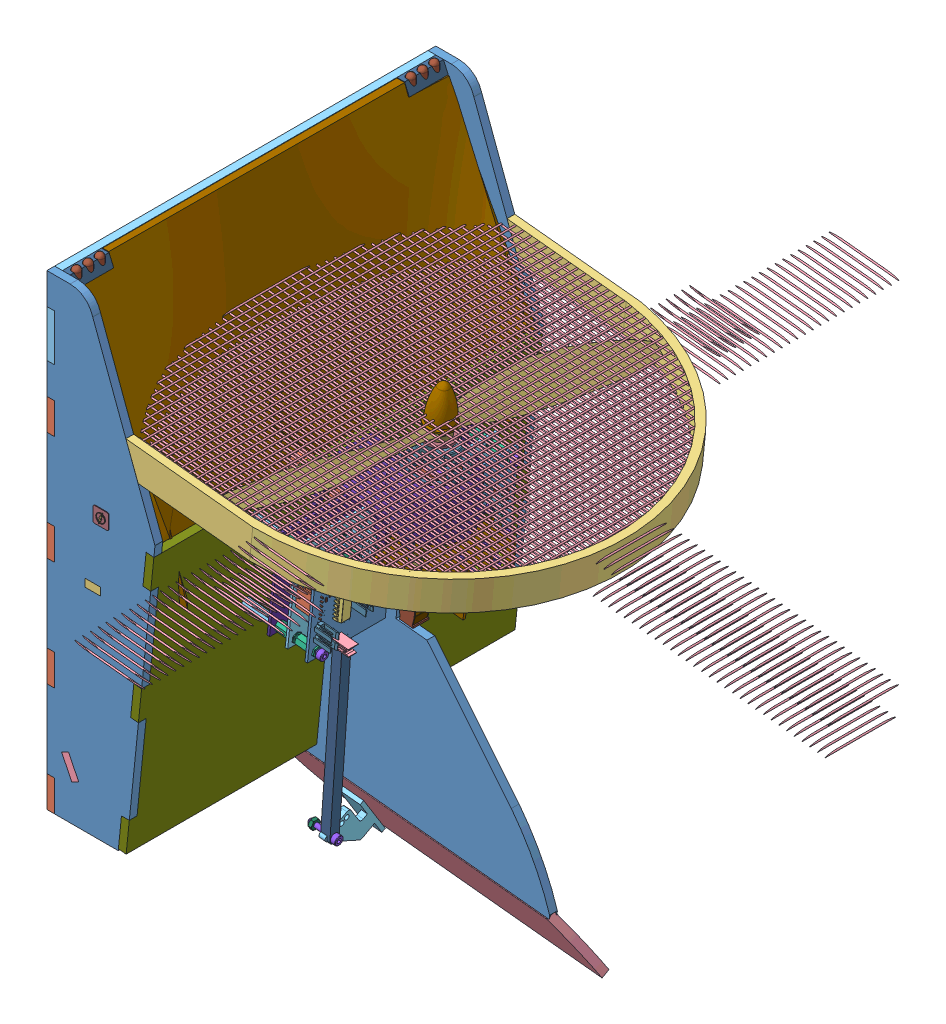
SolidWorks assembly AssTotaleSimu8, configuration Défaut. Lengths in mm.
Overall size (253.25 382.9 251.6).
1718 component instances, 230 part files, 11 mates.
Components (placement in the parent):
- AssStructSimu-1: AssStructSimu [Défaut] at (-125.7658 -1.8483 624.6548) x (1 0 0) z (0 0 -1) size (253.25 324.59 251.6)
  - AssBase-1: AssBase [Défaut] at (36.5482 -71.0398 34.0612) size (86.08 302.3 251.6)
    - AssD-1: AssD [Défaut] at (39.0992 31.0201 8.5) size (69.5 300 22)
      - P1-1: P1 [Défaut] at (-95.5819 194.6656 377.5) size (69.5 300 5)
      - P5-1: P5 [Défaut] at (-100.5819 -35.3344 360.5) x (0 1 0) z (1 0 0) size (230 22 5)
    - AssG-1: AssG [Défaut] at (39.0992 31.0201 -236.5) size (69.5 300 22)
      - P1-1: P1 [Défaut] at (-95.5819 194.6656 377.5) size (69.5 300 5)
      - P5-1: P5 [Défaut] at (-95.5819 -35.3344 399.5) x (0 1 0) z (-1 0 0) size (230 22 5)
    - P7-1: P7 [Défaut] at (-1.4828 89.6857 370.5) x (0 0 -1) z (0 -1 0) size (250 54.5 5)
    - P4-1: P4 [Défaut] at (-63.2363 165.9323 386) x (0 0 -1) z (0.898794 -0.438371 0) size (250 60.5 66.27)
    - P3-1: P3 [Défaut] at (-56.4828 -74.3143 146) x (0 0 1) z (-1 0 0) size (250 70 5)
    - P4b-1: P4b [Défaut] at (-58.7423 163.7404 190) x (0 0 1) z (0.438371 0.898794 0) size (152 56 2)
    - battery-1: battery [Défaut] at (-39.0156 204.1861 197.5) x (0 0 1) z (0.898794 -0.438371 0) size (137 43 30)
    - socket head cap screw 4762_din-1: socket head cap screw 4762_din [EN ISO 4762 M3 x 10 - 10N] at (-27.7008 145.2627 193) x (0.438371 0.898794 0) z (0 0 -1) size (13 5.5 5.5)
    - socket head cap screw 4762_din-2: socket head cap screw 4762_din [EN ISO 4762 M3 x 10 - 10N] at (-27.7008 145.2627 339) x (0.438371 0.898794 0) z (-0.791285 0.385936 -0.474259) size (13 5.5 5.5)
    - socket head cap screw 4762_din-3: socket head cap screw 4762_din [EN ISO 4762 M3 x 10 - 10N] at (-42.0815 152.2766 339) x (0.438371 0.898794 0) z (-0.001489 0.000726 -0.999999) size (13 5.5 5.5)
    - socket head cap screw 4762_din-4: socket head cap screw 4762_din [EN ISO 4762 M3 x 10 - 10N] at (-42.0815 152.2766 193) x (0.438371 0.898794 0) z (-0.031331 0.015281 -0.999392) size (13 5.5 5.5)
    - P11-1: P11 [Défaut] at (-57.5734 -73.9703 146.7843) x (0.005072 0 0.999987) z (0.006197 0.999981 -0.000031) size (240 65 164)
    - AssPhare-1: AssPhare [Défaut] at (-52.8518 -67.6977 411) x (0 1 0) z (0 0 -1) size (35.8 8 25)
      - piece_led-1: piece_led [Défaut] at (-6.6166 -3.631 25) size (7 8 25)
      - LED 5mm-1: LED 5mm [Valor predeterminado] at (-0.1166 0.369 30) x (0 0 1) z (-1 0 0) size (10.06 6 40.8)
      - LED 5mm-2: LED 5mm [Valor predeterminado] at (-0.1166 0.369 37.5) x (0 0 1) z (-1 0 0) size (10.06 6 40.8)
      - LED 5mm-3: LED 5mm [Valor predeterminado] at (-0.1166 0.369 45) x (0 0 1) z (-1 0 0) size (10.06 6 40.8)
    - AssPhare-2: AssPhare [Défaut] at (-52.8518 -67.6977 196) x (0 1 0) z (0 0 -1) size (35.8 8 25)
      - piece_led-1: piece_led [Défaut] at (-6.6166 -3.631 25) size (7 8 25)
      - LED 5mm-1: LED 5mm [Valor predeterminado] at (-0.1166 0.369 30) x (0 0 1) z (-1 0 0) size (10.06 6 40.8)
      - LED 5mm-2: LED 5mm [Valor predeterminado] at (-0.1166 0.369 37.5) x (0 0 1) z (-1 0 0) size (10.06 6 40.8)
      - LED 5mm-3: LED 5mm [Valor predeterminado] at (-0.1166 0.369 45) x (0 0 1) z (-1 0 0) size (10.06 6 40.8)
    - AssLogo-1: AssLogo [Défaut] at (-27.8835 45.1673 148.1054) x (-1 0 0) z (0 0 -1) size (10 10 0.8)
      - logo1-1: logo1 [Défaut] at (-6.5271 -4.4734 6.5054) size (5.8 7.71 0.4)
      - logo2-1: logo2 [Défaut] at (-6.4007 -4.4815 7.1054) size (10 10 0.4)
    - AssLogo-2: AssLogo [Défaut] at (-25.082 45.1673 383.8946) size (10 10 0.8)
      - logo1-1: logo1 [Défaut] at (-6.5271 -4.4734 6.5054) size (5.8 7.71 0.4)
      - logo2-1: logo2 [Défaut] at (-6.4007 -4.4815 7.1054) size (10 10 0.4)
    - support2-1: support2 [Défaut] at (-61.5648 191.7124 276) x (-0.017452 -0.999848 0) z (0.999848 -0.017452 0) size (75 20 10)
    - socket head cap screw 4762_din-5: socket head cap screw 4762_din [EN ISO 4762 M3 x 5 - 5N] at (-61.652 186.7132 269.3333) x (0.999848 -0.017452 0) z (-0.002158 -0.123615 0.992328) size (8 5.5 5.5)
    - socket head cap screw 4762_din-6: socket head cap screw 4762_din [EN ISO 4762 M3 x 5 - 5N] at (-61.652 186.7132 262.6667) x (0.999848 -0.017452 0) z (0 0 1) size (8 5.5 5.5)
    - socket head cap screw 4762_din-7: socket head cap screw 4762_din [EN ISO 4762 M3 x 25 - 18N] at (-55.2963 121.0922 253) x (0 0 1) z (-1 0 0) size (28 5.5 5.5)
    - hex nut style 1 gradeab_din-1: hex nut style 1 gradeab_din [Hexagon Nut ISO 4032 - M3 - W - N] at (-55.2963 121.0922 276) x (-0.923728 -0.383049 0) z (0 0 -1) size (5.5 6.35 2.4)
  - AssToitMot-1: AssToitMot [Défaut] at (-168.5238 43.6961 238.494) x (0 0 -1) z (0.9948 0.101852 0) size (250 207.5 205)
    - AssToit-1: AssToit [Défaut] at (-23.0702 -16.5789 -3.7148) size (250 207.5 205)
      - P8-1: P8 [Défaut] at (-38.4971 122.5921 203.5) size (250 175 5)
      - P12-1: P12 [Défaut] at (-60.4971 -63.4079 265.5) x (1 0 0) z (0 -1 0) size (47.03 76.64 55)
      - P13-1: P13 [Défaut] at (-35.9971 -52.8579 208.5) x (0 0 1) z (-1 0 0) size (64 15.55 5)
      - P10_2-1: P10_2 [Défaut] at (-35.9971 111.5921 171) x (0 0 1) z (-1 0 0) size (188.5 117.6 5)
    - Parallax-Servo_DUMMY-1: Parallax-Servo_DUMMY [Défaut] at (-61.6002 -51.5207 216.6662) x (1 0 0) z (0 1 0) size (20.07 42.67 55.64)
    - socket head cap screw 4762_din-1: socket head cap screw 4762_din [EN ISO 4762 M2.5 x 5 - 5N] at (-51.9272 -76.4868 259.2852) x (0 -1 0) z (-0.546944 0 0.837169) size (7.5 4.5 4.5)
    - socket head cap screw 4762_din-2: socket head cap screw 4762_din [EN ISO 4762 M2.5 x 5 - 5N] at (-61.5672 -76.4868 268.9252) x (0 -1 0) z (-0.546944 0 0.837169) size (7.5 4.5 4.5)
    - socket head cap screw 4762_din-3: socket head cap screw 4762_din [EN ISO 4762 M2.5 x 5 - 5N] at (-71.2072 -76.4868 259.2852) x (0 -1 0) z (-0.546944 0 0.837169) size (7.5 4.5 4.5)
    - socket head cap screw 4762_din-4: socket head cap screw 4762_din [EN ISO 4762 M2.5 x 5 - 5N] at (-61.5672 -76.4868 249.6452) x (0 -1 0) z (-0.546944 0 0.837169) size (7.5 4.5 4.5)
    - AssPhare-1: AssPhare [Défaut] at (8.4328 83.3966 196.1542) x (0 -1 0) z (1 0 0) size (35.8 8 25)
      - piece_led-1: piece_led [Défaut] at (-6.6166 -3.631 25) size (7 8 25)
      - LED 5mm-1: LED 5mm [Valor predeterminado] at (-0.1166 0.369 30) x (0 0 1) z (-1 0 0) size (10.06 6 40.8)
      - LED 5mm-2: LED 5mm [Valor predeterminado] at (-0.1166 0.369 37.5) x (0 0 1) z (-1 0 0) size (10.06 6 40.8)
      - LED 5mm-3: LED 5mm [Valor predeterminado] at (-0.1166 0.369 45) x (0 0 1) z (-1 0 0) size (10.06 6 40.8)
    - AssPhare-2: AssPhare [Défaut] at (-206.5672 83.3966 196.1542) x (0 -1 0) z (1 0 0) size (35.8 8 25)
      - piece_led-1: piece_led [Défaut] at (-6.6166 -3.631 25) size (7 8 25)
      - LED 5mm-1: LED 5mm [Valor predeterminado] at (-0.1166 0.369 30) x (0 0 1) z (-1 0 0) size (10.06 6 40.8)
      - LED 5mm-2: LED 5mm [Valor predeterminado] at (-0.1166 0.369 37.5) x (0 0 1) z (-1 0 0) size (10.06 6 40.8)
      - LED 5mm-3: LED 5mm [Valor predeterminado] at (-0.1166 0.369 45) x (0 0 1) z (-1 0 0) size (10.06 6 40.8)
    - socket head cap screw 4762_din-5: socket head cap screw 4762_din [EN ISO 4762 M3 x 10 - 10N] at (-67.0672 -22.9368 210.2852) x (0 0 -1) z (1 0 0) size (13 5.5 5.5)
    - socket head cap screw 4762_din-6: socket head cap screw 4762_din [EN ISO 4762 M3 x 10 - 10N] at (-56.0672 -72.9868 210.2852) x (0 0 -1) z (1 0 0) size (13 5.5 5.5)
    - socket head cap screw 4762_din-7: socket head cap screw 4762_din [EN ISO 4762 M3 x 10 - 10N] at (-67.0672 -72.9868 210.2852) x (0 0 -1) z (1 0 0) size (13 5.5 5.5)
    - socket head cap screw 4762_din-8: socket head cap screw 4762_din [EN ISO 4762 M3 x 10 - 10N] at (-56.0672 -22.9368 210.2852) x (0 0 -1) z (1 0 0) size (13 5.5 5.5)
    - hex nut style 1 gradeab_din-1: hex nut style 1 gradeab_din [Hexagon Nut ISO 4032 - M3 - W - N] at (-67.0672 -72.9868 197.3852) x (-0.923728 -0.383049 0) z (0 0 -1) size (5.5 6.35 2.4)
    - hex nut style 1 gradeab_din-2: hex nut style 1 gradeab_din [Hexagon Nut ISO 4032 - M3 - W - N] at (-56.0672 -72.9868 199.7852) size (5.5 6.35 2.4)
    - hex nut style 1 gradeab_din-3: hex nut style 1 gradeab_din [Hexagon Nut ISO 4032 - M3 - W - N] at (-67.0672 -22.9368 199.7852) size (5.5 6.35 2.4)
    - hex nut style 1 gradeab_din-4: hex nut style 1 gradeab_din [Hexagon Nut ISO 4032 - M3 - W - N] at (-56.0672 -22.9368 199.7852) size (5.5 6.35 2.4)
  - AssProtec-1: AssProtec [Défaut] at (86.6746 190.4649 284.6351) x (0 0 -1) z (0.101852 -0.9948 0) size (250 237.46 20)
    - protec3c-1: protec3c [Défaut] at (-140.4261 -87.7568 240) size (250 197 20)
    - AssGrillage-1: AssGrillage [Défaut] at (-370.4609 -132.5428 258.3161) x (0 0 -1) z (1 0 0) size (2.02 237.05 250)
      - barreau-1: barreau [Défaut] at (-1.1839 0.254 200) size (1 1 400)
      - barreau-3: barreau [Défaut] at (-1.1839 5.254 200) size (1 1 400)
      - barreau-4: barreau [Défaut] at (-1.1839 10.254 200) size (1 1 400)
      - barreau-5: barreau [Défaut] at (-1.1839 15.254 200) size (1 1 400)
      - barreau-6: barreau [Défaut] at (-1.1839 20.254 200) size (1 1 400)
      - barreau-7: barreau [Défaut] at (-1.1839 25.254 200) size (1 1 400)
      - barreau-8: barreau [Défaut] at (-1.1839 30.254 200) size (1 1 400)
      - barreau-9: barreau [Défaut] at (-1.1839 35.254 200) size (1 1 400)
      - barreau-10: barreau [Défaut] at (-1.1839 40.254 200) size (1 1 400)
      - barreau-11: barreau [Défaut] at (-1.1839 45.254 200) size (1 1 400)
      - barreau-12: barreau [Défaut] at (-1.1839 50.254 200) size (1 1 400)
      - barreau-13: barreau [Défaut] at (-1.1839 55.254 200) size (1 1 400)
      - barreau-14: barreau [Défaut] at (-1.1839 60.254 200) size (1 1 400)
      - barreau-15: barreau [Défaut] at (-1.1839 65.254 200) size (1 1 400)
      - barreau-16: barreau [Défaut] at (-1.1839 70.254 200) size (1 1 400)
      - barreau-17: barreau [Défaut] at (-1.1839 75.254 200) size (1 1 400)
      - barreau-18: barreau [Défaut] at (-1.1839 80.254 200) size (1 1 400)
      - barreau-19: barreau [Défaut] at (-1.1839 85.254 200) size (1 1 400)
      - barreau-20: barreau [Défaut] at (-1.1839 90.254 200) size (1 1 400)
      - barreau-21: barreau [Défaut] at (-1.1839 95.254 200) size (1 1 400)
      - barreau-22: barreau [Défaut] at (-1.1839 100.254 200) size (1 1 400)
      - barreau-23: barreau [Défaut] at (-1.1839 105.254 200) size (1 1 400)
      - barreau-24: barreau [Défaut] at (-1.1839 110.254 200) size (1 1 400)
      - barreau-25: barreau [Défaut] at (-1.1839 115.254 200) size (1 1 400)
      - barreau-26: barreau [Défaut] at (-1.1839 120.254 200) size (1 1 400)
      - barreau-27: barreau [Défaut] at (-1.1839 125.254 200) size (1 1 400)
      - barreau-28: barreau [Défaut] at (-1.1839 130.254 200) size (1 1 400)
      - barreau-29: barreau [Défaut] at (-1.1839 135.254 200) size (1 1 400)
      - barreau-30: barreau [Défaut] at (-1.1839 140.254 200) size (1 1 400)
      - barreau-31: barreau [Défaut] at (-1.1839 145.254 200) size (1 1 400)
      - barreau-32: barreau [Défaut] at (-1.1839 150.254 200) size (1 1 400)
      - barreau-33: barreau [Défaut] at (-1.1839 155.254 200) size (1 1 400)
      - barreau-34: barreau [Défaut] at (-1.1839 160.254 200) size (1 1 400)
      - barreau-35: barreau [Défaut] at (-1.1839 165.254 200) size (1 1 400)
      - barreau-36: barreau [Défaut] at (-1.1839 170.254 200) size (1 1 400)
      - barreau-37: barreau [Défaut] at (-1.1839 175.254 200) size (1 1 400)
      - barreau-38: barreau [Défaut] at (-1.1839 180.254 200) size (1 1 400)
      - barreau-39: barreau [Défaut] at (-1.1839 185.254 200) size (1 1 400)
      - barreau-40: barreau [Défaut] at (-1.1839 190.254 200) size (1 1 400)
      - barreau-41: barreau [Défaut] at (-1.1839 195.254 200) size (1 1 400)
      - barreau-42: barreau [Défaut] at (-0.1839 -1.5314 598.7823) x (0.998922 0 0.04641) z (0 1 0) size (1 1 400)
      - barreau-43: barreau [Défaut] at (-1.1839 200.254 200) size (1 1 400)
      - barreau-44: barreau [Défaut] at (-1.1839 205.254 200) size (1 1 400)
      - barreau-45: barreau [Défaut] at (-1.1839 210.254 200) size (1 1 400)
      - barreau-46: barreau [Défaut] at (-1.1839 215.254 200) size (1 1 400)
      - barreau-47: barreau [Défaut] at (-1.1839 220.254 200) size (1 1 400)
      - barreau-48: barreau [Défaut] at (-1.1839 225.254 200) size (1 1 400)
      - barreau-49: barreau [Défaut] at (-1.1839 230.254 200) size (1 1 400)
      - barreau-50: barreau [Défaut] at (-1.1839 235.254 200) size (1 1 400)
      - barreau-51: barreau [Défaut] at (-1.1839 240.254 200) size (1 1 400)
      - barreau-52: barreau [Défaut] at (-1.1839 245.254 200) size (1 1 400)
      - barreau-53: barreau [Défaut] at (-1.1839 250.254 200) size (1 1 400)
      - barreau-54: barreau [Défaut] at (-1.1839 255.254 200) size (1 1 400)
      - barreau-55: barreau [Défaut] at (-1.1839 260.254 200) size (1 1 400)
      - barreau-56: barreau [Défaut] at (-1.1839 265.254 200) size (1 1 400)
      - barreau-57: barreau [Défaut] at (-1.1839 270.254 200) size (1 1 400)
      - barreau-58: barreau [Défaut] at (-1.1839 275.254 200) size (1 1 400)
      - barreau-59: barreau [Défaut] at (-1.1839 280.254 200) size (1 1 400)
      - barreau-60: barreau [Défaut] at (-1.1839 285.254 200) size (1 1 400)
      - barreau-61: barreau [Défaut] at (-1.1839 290.254 200) size (1 1 400)
      - barreau-62: barreau [Défaut] at (-1.1839 295.254 200) size (1 1 400)
      - barreau-63: barreau [Défaut] at (-1.1839 300.254 200) size (1 1 400)
      - barreau-64: barreau [Défaut] at (-1.1839 305.254 200) size (1 1 400)
      - barreau-65: barreau [Défaut] at (-1.1839 310.254 200) size (1 1 400)
      - barreau-66: barreau [Défaut] at (-1.1839 315.254 200) size (1 1 400)
      - barreau-67: barreau [Défaut] at (-1.1839 320.254 200) size (1 1 400)
      - barreau-68: barreau [Défaut] at (-1.1839 325.254 200) size (1 1 400)
      - barreau-69: barreau [Défaut] at (-1.1839 330.254 200) size (1 1 400)
      - barreau-70: barreau [Défaut] at (-1.1839 335.254 200) size (1 1 400)
      - barreau-71: barreau [Défaut] at (-1.1839 340.254 200) size (1 1 400)
      - barreau-72: barreau [Défaut] at (-1.1839 345.254 200) size (1 1 400)
      - barreau-73: barreau [Défaut] at (-1.1839 350.254 200) size (1 1 400)
      - barreau-74: barreau [Défaut] at (-1.1839 355.254 200) size (1 1 400)
      - barreau-75: barreau [Défaut] at (-1.1839 360.254 200) size (1 1 400)
      - barreau-76: barreau [Défaut] at (-1.1839 365.254 200) size (1 1 400)
      - barreau-77: barreau [Défaut] at (-1.1839 370.254 200) size (1 1 400)
      - barreau-78: barreau [Défaut] at (-1.1839 375.254 200) size (1 1 400)
      - barreau-79: barreau [Défaut] at (-1.1839 380.254 200) size (1 1 400)
      - barreau-80: barreau [Défaut] at (-1.1839 385.254 200) size (1 1 400)
      - barreau-81: barreau [Défaut] at (-1.1839 390.254 200) size (1 1 400)
      - barreau-82: barreau [Défaut] at (-1.1839 395.254 200) size (1 1 400)
      - barreau-136: barreau [Défaut] at (-0.1839 -1.5314 593.7823) x (0.998922 0 0.04641) z (0 1 0) size (1 1 400)
      - barreau-137: barreau [Défaut] at (-0.1839 -1.5314 588.7823) x (0.998922 0 0.04641) z (0 1 0) size (1 1 400)
      - barreau-138: barreau [Défaut] at (-0.1839 -1.5314 583.7823) x (0.998922 0 0.04641) z (0 1 0) size (1 1 400)
      - barreau-139: barreau [Défaut] at (-0.1839 -1.5314 578.7823) x (0.998922 0 0.04641) z (0 1 0) size (1 1 400)
      - barreau-140: barreau [Défaut] at (-0.1839 -1.5314 573.7823) x (0.998922 0 0.04641) z (0 1 0) size (1 1 400)
      - barreau-141: barreau [Défaut] at (-0.1839 -1.5314 568.7823) x (0.998922 0 0.04641) z (0 1 0) size (1 1 400)
      - barreau-142: barreau [Défaut] at (-0.1839 -1.5314 563.7823) x (0.998922 0 0.04641) z (0 1 0) size (1 1 400)
      - barreau-143: barreau [Défaut] at (-0.1839 -1.5314 558.7823) x (0.998922 0 0.04641) z (0 1 0) size (1 1 400)
      - barreau-144: barreau [Défaut] at (-0.1839 -1.5314 553.7823) x (0.998922 0 0.04641) z (0 1 0) size (1 1 400)
      - barreau-145: barreau [Défaut] at (-0.1839 -1.5314 548.7823) x (0.998922 0 0.04641) z (0 1 0) size (1 1 400)
      - barreau-146: barreau [Défaut] at (-0.1839 -1.5314 543.7823) x (0.998922 0 0.04641) z (0 1 0) size (1 1 400)
      - barreau-147: barreau [Défaut] at (-0.1839 -1.5314 538.7823) x (0.998922 0 0.04641) z (0 1 0) size (1 1 400)
      - barreau-148: barreau [Défaut] at (-0.1839 -1.5314 533.7823) x (0.998922 0 0.04641) z (0 1 0) size (1 1 400)
      - barreau-149: barreau [Défaut] at (-0.1839 -1.5314 528.7823) x (0.998922 0 0.04641) z (0 1 0) size (1 1 400)
      - barreau-150: barreau [Défaut] at (-0.1839 -1.5314 523.7823) x (0.998922 0 0.04641) z (0 1 0) size (1 1 400)
      - barreau-151: barreau [Défaut] at (-0.1839 -1.5314 518.7823) x (0.998922 0 0.04641) z (0 1 0) size (1 1 400)
      - barreau-152: barreau [Défaut] at (-0.1839 -1.5314 513.7823) x (0.998922 0 0.04641) z (0 1 0) size (1 1 400)
      - barreau-153: barreau [Défaut] at (-0.1839 -1.5314 508.7823) x (0.998922 0 0.04641) z (0 1 0) size (1 1 400)
      - barreau-154: barreau [Défaut] at (-0.1839 -1.5314 503.7823) x (0.998922 0 0.04641) z (0 1 0) size (1 1 400)
      - barreau-155: barreau [Défaut] at (-0.1839 -1.5314 498.7823) x (0.998922 0 0.04641) z (0 1 0) size (1 1 400)
      - barreau-156: barreau [Défaut] at (-0.1839 -1.5314 493.7823) x (0.998922 0 0.04641) z (0 1 0) size (1 1 400)
      - barreau-157: barreau [Défaut] at (-0.1839 -1.5314 488.7823) x (0.998922 0 0.04641) z (0 1 0) size (1 1 400)
      - barreau-158: barreau [Défaut] at (-0.1839 -1.5314 483.7823) x (0.998922 0 0.04641) z (0 1 0) size (1 1 400)
      - barreau-159: barreau [Défaut] at (-0.1839 -1.5314 478.7823) x (0.998922 0 0.04641) z (0 1 0) size (1 1 400)
      - barreau-160: barreau [Défaut] at (-0.1839 -1.5314 473.7823) x (0.998922 0 0.04641) z (0 1 0) size (1 1 400)
      - barreau-161: barreau [Défaut] at (-0.1839 -1.5314 468.7823) x (0.998922 0 0.04641) z (0 1 0) size (1 1 400)
      - barreau-162: barreau [Défaut] at (-0.1839 -1.5314 463.7823) x (0.998922 0 0.04641) z (0 1 0) size (1 1 400)
      - barreau-163: barreau [Défaut] at (-0.1839 -1.5314 458.7823) x (0.998922 0 0.04641) z (0 1 0) size (1 1 400)
      - barreau-164: barreau [Défaut] at (-0.1839 -1.5314 453.7823) x (0.998922 0 0.04641) z (0 1 0) size (1 1 400)
      - barreau-165: barreau [Défaut] at (-0.1839 -1.5314 448.7823) x (0.998922 0 0.04641) z (0 1 0) size (1 1 400)
      - barreau-166: barreau [Défaut] at (-0.1839 -1.5314 443.7823) x (0.998922 0 0.04641) z (0 1 0) size (1 1 400)
      - barreau-167: barreau [Défaut] at (-0.1839 -1.5314 438.7823) x (0.998922 0 0.04641) z (0 1 0) size (1 1 400)
      - barreau-168: barreau [Défaut] at (-0.1839 -1.5314 433.7823) x (0.998922 0 0.04641) z (0 1 0) size (1 1 400)
      - barreau-169: barreau [Défaut] at (-0.1839 -1.5314 428.7823) x (0.998922 0 0.04641) z (0 1 0) size (1 1 400)
      - barreau-170: barreau [Défaut] at (-0.1839 -1.5314 423.7823) x (0.998922 0 0.04641) z (0 1 0) size (1 1 400)
      - barreau-171: barreau [Défaut] at (-0.1839 -1.5314 418.7823) x (0.998922 0 0.04641) z (0 1 0) size (1 1 400)
      - barreau-172: barreau [Défaut] at (-0.1839 -1.5314 413.7823) x (0.998922 0 0.04641) z (0 1 0) size (1 1 400)
      - barreau-173: barreau [Défaut] at (-0.1839 -1.5314 408.7823) x (0.998922 0 0.04641) z (0 1 0) size (1 1 400)
      - barreau-174: barreau [Défaut] at (-0.1839 -1.5314 403.7823) x (0.998922 0 0.04641) z (0 1 0) size (1 1 400)
      - barreau-175: barreau [Défaut] at (-0.1839 -1.5314 398.7823) x (0.998922 0 0.04641) z (0 1 0) size (1 1 400)
      - barreau-176: barreau [Défaut] at (-0.1839 -1.5314 393.7823) x (0.998922 0 0.04641) z (0 1 0) size (1 1 400)
      - barreau-177: barreau [Défaut] at (-0.1839 -1.5314 388.7823) x (0.998922 0 0.04641) z (0 1 0) size (1 1 400)
      - barreau-178: barreau [Défaut] at (-0.1839 -1.5314 383.7823) x (0.998922 0 0.04641) z (0 1 0) size (1 1 400)
      - barreau-179: barreau [Défaut] at (-0.1839 -1.5314 378.7823) x (0.998922 0 0.04641) z (0 1 0) size (1 1 400)
      - barreau-180: barreau [Défaut] at (-0.1839 -1.5314 373.7823) x (0.998922 0 0.04641) z (0 1 0) size (1 1 400)
      - barreau-181: barreau [Défaut] at (-0.1839 -1.5314 368.7823) x (0.998922 0 0.04641) z (0 1 0) size (1 1 400)
      - barreau-182: barreau [Défaut] at (-0.1839 -1.5314 363.7823) x (0.998922 0 0.04641) z (0 1 0) size (1 1 400)
      - barreau-183: barreau [Défaut] at (-0.1839 -1.5314 358.7823) x (0.998922 0 0.04641) z (0 1 0) size (1 1 400)
      - barreau-184: barreau [Défaut] at (-0.1839 -1.5314 353.7823) x (0.998922 0 0.04641) z (0 1 0) size (1 1 400)
      - barreau-185: barreau [Défaut] at (-0.1839 -1.5314 348.7823) x (0.998922 0 0.04641) z (0 1 0) size (1 1 400)
      - barreau-186: barreau [Défaut] at (-0.1839 -1.5314 343.7823) x (0.998922 0 0.04641) z (0 1 0) size (1 1 400)
      - barreau-187: barreau [Défaut] at (-0.1839 -1.5314 338.7823) x (0.998922 0 0.04641) z (0 1 0) size (1 1 400)
      - barreau-188: barreau [Défaut] at (-0.1839 -1.5314 333.7823) x (0.998922 0 0.04641) z (0 1 0) size (1 1 400)
      - barreau-189: barreau [Défaut] at (-0.1839 -1.5314 328.7823) x (0.998922 0 0.04641) z (0 1 0) size (1 1 400)
      - barreau-190: barreau [Défaut] at (-0.1839 -1.5314 323.7823) x (0.998922 0 0.04641) z (0 1 0) size (1 1 400)
      - barreau-191: barreau [Défaut] at (-0.1839 -1.5314 318.7823) x (0.998922 0 0.04641) z (0 1 0) size (1 1 400)
      - barreau-192: barreau [Défaut] at (-0.1839 -1.5314 313.7823) x (0.998922 0 0.04641) z (0 1 0) size (1 1 400)
      - barreau-193: barreau [Défaut] at (-0.1839 -1.5314 308.7823) x (0.998922 0 0.04641) z (0 1 0) size (1 1 400)
      - barreau-194: barreau [Défaut] at (-0.1839 -1.5314 303.7823) x (0.998922 0 0.04641) z (0 1 0) size (1 1 400)
      - barreau-195: barreau [Défaut] at (-0.1839 -1.5314 298.7823) x (0.998922 0 0.04641) z (0 1 0) size (1 1 400)
      - barreau-196: barreau [Défaut] at (-0.1839 -1.5314 293.7823) x (0.998922 0 0.04641) z (0 1 0) size (1 1 400)
      - barreau-197: barreau [Défaut] at (-0.1839 -1.5314 288.7823) x (0.998922 0 0.04641) z (0 1 0) size (1 1 400)
      - barreau-198: barreau [Défaut] at (-0.1839 -1.5314 283.7823) x (0.998922 0 0.04641) z (0 1 0) size (1 1 400)
      - barreau-199: barreau [Défaut] at (-0.1839 -1.5314 278.7823) x (0.998922 0 0.04641) z (0 1 0) size (1 1 400)
      - barreau-200: barreau [Défaut] at (-0.1839 -1.5314 273.7823) x (0.998922 0 0.04641) z (0 1 0) size (1 1 400)
      - barreau-201: barreau [Défaut] at (-0.1839 -1.5314 268.7823) x (0.998922 0 0.04641) z (0 1 0) size (1 1 400)
      - barreau-202: barreau [Défaut] at (-0.1839 -1.5314 263.7823) x (0.998922 0 0.04641) z (0 1 0) size (1 1 400)
      - barreau-203: barreau [Défaut] at (-0.1839 -1.5314 258.7823) x (0.998922 0 0.04641) z (0 1 0) size (1 1 400)
      - barreau-204: barreau [Défaut] at (-0.1839 -1.5314 253.7823) x (0.998922 0 0.04641) z (0 1 0) size (1 1 400)
      - barreau-205: barreau [Défaut] at (-0.1839 -1.5314 248.7823) x (0.998922 0 0.04641) z (0 1 0) size (1 1 400)
      - barreau-206: barreau [Défaut] at (-0.1839 -1.5314 243.7823) x (0.998922 0 0.04641) z (0 1 0) size (1 1 400)
      - barreau-207: barreau [Défaut] at (-0.1839 -1.5314 238.7823) x (0.998922 0 0.04641) z (0 1 0) size (1 1 400)
      - barreau-208: barreau [Défaut] at (-0.1839 -1.5314 233.7823) x (0.998922 0 0.04641) z (0 1 0) size (1 1 400)
      - barreau-209: barreau [Défaut] at (-0.1839 -1.5314 228.7823) x (0.998922 0 0.04641) z (0 1 0) size (1 1 400)
      - barreau-210: barreau [Défaut] at (-0.1839 -1.5314 223.7823) x (0.998922 0 0.04641) z (0 1 0) size (1 1 400)
      - barreau-211: barreau [Défaut] at (-0.1839 -1.5314 218.7823) x (0.998922 0 0.04641) z (0 1 0) size (1 1 400)
      - barreau-212: barreau [Défaut] at (-0.1839 -1.5314 213.7823) x (0.998922 0 0.04641) z (0 1 0) size (1 1 400)
      - barreau-213: barreau [Défaut] at (-0.1839 -1.5314 208.7823) x (0.998922 0 0.04641) z (0 1 0) size (1 1 400)
      - barreau-214: barreau [Défaut] at (-0.1839 -1.5314 203.7823) x (0.998922 0 0.04641) z (0 1 0) size (1 1 400)
    - AssGrillage-2: AssGrillage [Défaut] at (339.6086 -132.5428 241.6839) x (0 0 1) z (-1 0 0) size (2.02 237.05 250)
      - barreau-1: barreau [Défaut] at (-1.1839 0.254 200) size (1 1 400)
      - barreau-3: barreau [Défaut] at (-1.1839 5.254 200) size (1 1 400)
      - barreau-4: barreau [Défaut] at (-1.1839 10.254 200) size (1 1 400)
      - barreau-5: barreau [Défaut] at (-1.1839 15.254 200) size (1 1 400)
      - barreau-6: barreau [Défaut] at (-1.1839 20.254 200) size (1 1 400)
      - barreau-7: barreau [Défaut] at (-1.1839 25.254 200) size (1 1 400)
      - barreau-8: barreau [Défaut] at (-1.1839 30.254 200) size (1 1 400)
      - barreau-9: barreau [Défaut] at (-1.1839 35.254 200) size (1 1 400)
      - barreau-10: barreau [Défaut] at (-1.1839 40.254 200) size (1 1 400)
      - barreau-11: barreau [Défaut] at (-1.1839 45.254 200) size (1 1 400)
      - barreau-12: barreau [Défaut] at (-1.1839 50.254 200) size (1 1 400)
      - barreau-13: barreau [Défaut] at (-1.1839 55.254 200) size (1 1 400)
      - barreau-14: barreau [Défaut] at (-1.1839 60.254 200) size (1 1 400)
      - barreau-15: barreau [Défaut] at (-1.1839 65.254 200) size (1 1 400)
      - barreau-16: barreau [Défaut] at (-1.1839 70.254 200) size (1 1 400)
      - barreau-17: barreau [Défaut] at (-1.1839 75.254 200) size (1 1 400)
      - barreau-18: barreau [Défaut] at (-1.1839 80.254 200) size (1 1 400)
      - barreau-19: barreau [Défaut] at (-1.1839 85.254 200) size (1 1 400)
      - barreau-20: barreau [Défaut] at (-1.1839 90.254 200) size (1 1 400)
      - barreau-21: barreau [Défaut] at (-1.1839 95.254 200) size (1 1 400)
      - barreau-22: barreau [Défaut] at (-1.1839 100.254 200) size (1 1 400)
      - barreau-23: barreau [Défaut] at (-1.1839 105.254 200) size (1 1 400)
      - barreau-24: barreau [Défaut] at (-1.1839 110.254 200) size (1 1 400)
      - barreau-25: barreau [Défaut] at (-1.1839 115.254 200) size (1 1 400)
      - barreau-26: barreau [Défaut] at (-1.1839 120.254 200) size (1 1 400)
      - barreau-27: barreau [Défaut] at (-1.1839 125.254 200) size (1 1 400)
      - barreau-28: barreau [Défaut] at (-1.1839 130.254 200) size (1 1 400)
      - barreau-29: barreau [Défaut] at (-1.1839 135.254 200) size (1 1 400)
      - barreau-30: barreau [Défaut] at (-1.1839 140.254 200) size (1 1 400)
      - barreau-31: barreau [Défaut] at (-1.1839 145.254 200) size (1 1 400)
      - barreau-32: barreau [Défaut] at (-1.1839 150.254 200) size (1 1 400)
      - barreau-33: barreau [Défaut] at (-1.1839 155.254 200) size (1 1 400)
      - barreau-34: barreau [Défaut] at (-1.1839 160.254 200) size (1 1 400)
      - barreau-35: barreau [Défaut] at (-1.1839 165.254 200) size (1 1 400)
      - barreau-36: barreau [Défaut] at (-1.1839 170.254 200) size (1 1 400)
      - barreau-37: barreau [Défaut] at (-1.1839 175.254 200) size (1 1 400)
      - barreau-38: barreau [Défaut] at (-1.1839 180.254 200) size (1 1 400)
      - barreau-39: barreau [Défaut] at (-1.1839 185.254 200) size (1 1 400)
      - barreau-40: barreau [Défaut] at (-1.1839 190.254 200) size (1 1 400)
      - barreau-41: barreau [Défaut] at (-1.1839 195.254 200) size (1 1 400)
      - barreau-42: barreau [Défaut] at (-0.1839 -1.5314 598.7823) x (0.998922 0 0.04641) z (0 1 0) size (1 1 400)
      - barreau-43: barreau [Défaut] at (-1.1839 200.254 200) size (1 1 400)
      - barreau-44: barreau [Défaut] at (-1.1839 205.254 200) size (1 1 400)
      - barreau-45: barreau [Défaut] at (-1.1839 210.254 200) size (1 1 400)
      - barreau-46: barreau [Défaut] at (-1.1839 215.254 200) size (1 1 400)
      - barreau-47: barreau [Défaut] at (-1.1839 220.254 200) size (1 1 400)
      - barreau-48: barreau [Défaut] at (-1.1839 225.254 200) size (1 1 400)
      - barreau-49: barreau [Défaut] at (-1.1839 230.254 200) size (1 1 400)
      - barreau-50: barreau [Défaut] at (-1.1839 235.254 200) size (1 1 400)
      - barreau-51: barreau [Défaut] at (-1.1839 240.254 200) size (1 1 400)
      - barreau-52: barreau [Défaut] at (-1.1839 245.254 200) size (1 1 400)
      - barreau-53: barreau [Défaut] at (-1.1839 250.254 200) size (1 1 400)
      - barreau-54: barreau [Défaut] at (-1.1839 255.254 200) size (1 1 400)
      - barreau-55: barreau [Défaut] at (-1.1839 260.254 200) size (1 1 400)
      - barreau-56: barreau [Défaut] at (-1.1839 265.254 200) size (1 1 400)
      - barreau-57: barreau [Défaut] at (-1.1839 270.254 200) size (1 1 400)
      - barreau-58: barreau [Défaut] at (-1.1839 275.254 200) size (1 1 400)
      - barreau-59: barreau [Défaut] at (-1.1839 280.254 200) size (1 1 400)
      - barreau-60: barreau [Défaut] at (-1.1839 285.254 200) size (1 1 400)
      - barreau-61: barreau [Défaut] at (-1.1839 290.254 200) size (1 1 400)
      - barreau-62: barreau [Défaut] at (-1.1839 295.254 200) size (1 1 400)
      - barreau-63: barreau [Défaut] at (-1.1839 300.254 200) size (1 1 400)
      - barreau-64: barreau [Défaut] at (-1.1839 305.254 200) size (1 1 400)
      - barreau-65: barreau [Défaut] at (-1.1839 310.254 200) size (1 1 400)
      - barreau-66: barreau [Défaut] at (-1.1839 315.254 200) size (1 1 400)
      - barreau-67: barreau [Défaut] at (-1.1839 320.254 200) size (1 1 400)
      - barreau-68: barreau [Défaut] at (-1.1839 325.254 200) size (1 1 400)
      - barreau-69: barreau [Défaut] at (-1.1839 330.254 200) size (1 1 400)
      - barreau-70: barreau [Défaut] at (-1.1839 335.254 200) size (1 1 400)
      - barreau-71: barreau [Défaut] at (-1.1839 340.254 200) size (1 1 400)
      - barreau-72: barreau [Défaut] at (-1.1839 345.254 200) size (1 1 400)
      - barreau-73: barreau [Défaut] at (-1.1839 350.254 200) size (1 1 400)
      - barreau-74: barreau [Défaut] at (-1.1839 355.254 200) size (1 1 400)
      - barreau-75: barreau [Défaut] at (-1.1839 360.254 200) size (1 1 400)
      - barreau-76: barreau [Défaut] at (-1.1839 365.254 200) size (1 1 400)
      - barreau-77: barreau [Défaut] at (-1.1839 370.254 200) size (1 1 400)
      - barreau-78: barreau [Défaut] at (-1.1839 375.254 200) size (1 1 400)
      - barreau-79: barreau [Défaut] at (-1.1839 380.254 200) size (1 1 400)
      - barreau-80: barreau [Défaut] at (-1.1839 385.254 200) size (1 1 400)
      - barreau-81: barreau [Défaut] at (-1.1839 390.254 200) size (1 1 400)
      - barreau-82: barreau [Défaut] at (-1.1839 395.254 200) size (1 1 400)
      - barreau-136: barreau [Défaut] at (-0.1839 -1.5314 593.7823) x (0.998922 0 0.04641) z (0 1 0) size (1 1 400)
      - barreau-137: barreau [Défaut] at (-0.1839 -1.5314 588.7823) x (0.998922 0 0.04641) z (0 1 0) size (1 1 400)
      - barreau-138: barreau [Défaut] at (-0.1839 -1.5314 583.7823) x (0.998922 0 0.04641) z (0 1 0) size (1 1 400)
      - barreau-139: barreau [Défaut] at (-0.1839 -1.5314 578.7823) x (0.998922 0 0.04641) z (0 1 0) size (1 1 400)
      - barreau-140: barreau [Défaut] at (-0.1839 -1.5314 573.7823) x (0.998922 0 0.04641) z (0 1 0) size (1 1 400)
      - barreau-141: barreau [Défaut] at (-0.1839 -1.5314 568.7823) x (0.998922 0 0.04641) z (0 1 0) size (1 1 400)
      - barreau-142: barreau [Défaut] at (-0.1839 -1.5314 563.7823) x (0.998922 0 0.04641) z (0 1 0) size (1 1 400)
      - barreau-143: barreau [Défaut] at (-0.1839 -1.5314 558.7823) x (0.998922 0 0.04641) z (0 1 0) size (1 1 400)
      - barreau-144: barreau [Défaut] at (-0.1839 -1.5314 553.7823) x (0.998922 0 0.04641) z (0 1 0) size (1 1 400)
      - barreau-145: barreau [Défaut] at (-0.1839 -1.5314 548.7823) x (0.998922 0 0.04641) z (0 1 0) size (1 1 400)
      - barreau-146: barreau [Défaut] at (-0.1839 -1.5314 543.7823) x (0.998922 0 0.04641) z (0 1 0) size (1 1 400)
      - barreau-147: barreau [Défaut] at (-0.1839 -1.5314 538.7823) x (0.998922 0 0.04641) z (0 1 0) size (1 1 400)
      - barreau-148: barreau [Défaut] at (-0.1839 -1.5314 533.7823) x (0.998922 0 0.04641) z (0 1 0) size (1 1 400)
      - barreau-149: barreau [Défaut] at (-0.1839 -1.5314 528.7823) x (0.998922 0 0.04641) z (0 1 0) size (1 1 400)
      - barreau-150: barreau [Défaut] at (-0.1839 -1.5314 523.7823) x (0.998922 0 0.04641) z (0 1 0) size (1 1 400)
      - barreau-151: barreau [Défaut] at (-0.1839 -1.5314 518.7823) x (0.998922 0 0.04641) z (0 1 0) size (1 1 400)
      - barreau-152: barreau [Défaut] at (-0.1839 -1.5314 513.7823) x (0.998922 0 0.04641) z (0 1 0) size (1 1 400)
      - barreau-153: barreau [Défaut] at (-0.1839 -1.5314 508.7823) x (0.998922 0 0.04641) z (0 1 0) size (1 1 400)
      - barreau-154: barreau [Défaut] at (-0.1839 -1.5314 503.7823) x (0.998922 0 0.04641) z (0 1 0) size (1 1 400)
      - barreau-155: barreau [Défaut] at (-0.1839 -1.5314 498.7823) x (0.998922 0 0.04641) z (0 1 0) size (1 1 400)
      - barreau-156: barreau [Défaut] at (-0.1839 -1.5314 493.7823) x (0.998922 0 0.04641) z (0 1 0) size (1 1 400)
      - barreau-157: barreau [Défaut] at (-0.1839 -1.5314 488.7823) x (0.998922 0 0.04641) z (0 1 0) size (1 1 400)
      - barreau-158: barreau [Défaut] at (-0.1839 -1.5314 483.7823) x (0.998922 0 0.04641) z (0 1 0) size (1 1 400)
      - barreau-159: barreau [Défaut] at (-0.1839 -1.5314 478.7823) x (0.998922 0 0.04641) z (0 1 0) size (1 1 400)
      - barreau-160: barreau [Défaut] at (-0.1839 -1.5314 473.7823) x (0.998922 0 0.04641) z (0 1 0) size (1 1 400)
      - barreau-161: barreau [Défaut] at (-0.1839 -1.5314 468.7823) x (0.998922 0 0.04641) z (0 1 0) size (1 1 400)
      - barreau-162: barreau [Défaut] at (-0.1839 -1.5314 463.7823) x (0.998922 0 0.04641) z (0 1 0) size (1 1 400)
      - barreau-163: barreau [Défaut] at (-0.1839 -1.5314 458.7823) x (0.998922 0 0.04641) z (0 1 0) size (1 1 400)
      - barreau-164: barreau [Défaut] at (-0.1839 -1.5314 453.7823) x (0.998922 0 0.04641) z (0 1 0) size (1 1 400)
      - barreau-165: barreau [Défaut] at (-0.1839 -1.5314 448.7823) x (0.998922 0 0.04641) z (0 1 0) size (1 1 400)
      - barreau-166: barreau [Défaut] at (-0.1839 -1.5314 443.7823) x (0.998922 0 0.04641) z (0 1 0) size (1 1 400)
      - barreau-167: barreau [Défaut] at (-0.1839 -1.5314 438.7823) x (0.998922 0 0.04641) z (0 1 0) size (1 1 400)
      - barreau-168: barreau [Défaut] at (-0.1839 -1.5314 433.7823) x (0.998922 0 0.04641) z (0 1 0) size (1 1 400)
      - barreau-169: barreau [Défaut] at (-0.1839 -1.5314 428.7823) x (0.998922 0 0.04641) z (0 1 0) size (1 1 400)
      - barreau-170: barreau [Défaut] at (-0.1839 -1.5314 423.7823) x (0.998922 0 0.04641) z (0 1 0) size (1 1 400)
      - barreau-171: barreau [Défaut] at (-0.1839 -1.5314 418.7823) x (0.998922 0 0.04641) z (0 1 0) size (1 1 400)
      - barreau-172: barreau [Défaut] at (-0.1839 -1.5314 413.7823) x (0.998922 0 0.04641) z (0 1 0) size (1 1 400)
      - barreau-173: barreau [Défaut] at (-0.1839 -1.5314 408.7823) x (0.998922 0 0.04641) z (0 1 0) size (1 1 400)
      - barreau-174: barreau [Défaut] at (-0.1839 -1.5314 403.7823) x (0.998922 0 0.04641) z (0 1 0) size (1 1 400)
      - barreau-175: barreau [Défaut] at (-0.1839 -1.5314 398.7823) x (0.998922 0 0.04641) z (0 1 0) size (1 1 400)
      - barreau-176: barreau [Défaut] at (-0.1839 -1.5314 393.7823) x (0.998922 0 0.04641) z (0 1 0) size (1 1 400)
      - barreau-177: barreau [Défaut] at (-0.1839 -1.5314 388.7823) x (0.998922 0 0.04641) z (0 1 0) size (1 1 400)
      - barreau-178: barreau [Défaut] at (-0.1839 -1.5314 383.7823) x (0.998922 0 0.04641) z (0 1 0) size (1 1 400)
      - barreau-179: barreau [Défaut] at (-0.1839 -1.5314 378.7823) x (0.998922 0 0.04641) z (0 1 0) size (1 1 400)
      - barreau-180: barreau [Défaut] at (-0.1839 -1.5314 373.7823) x (0.998922 0 0.04641) z (0 1 0) size (1 1 400)
      - barreau-181: barreau [Défaut] at (-0.1839 -1.5314 368.7823) x (0.998922 0 0.04641) z (0 1 0) size (1 1 400)
      - barreau-182: barreau [Défaut] at (-0.1839 -1.5314 363.7823) x (0.998922 0 0.04641) z (0 1 0) size (1 1 400)
      - barreau-183: barreau [Défaut] at (-0.1839 -1.5314 358.7823) x (0.998922 0 0.04641) z (0 1 0) size (1 1 400)
      - barreau-184: barreau [Défaut] at (-0.1839 -1.5314 353.7823) x (0.998922 0 0.04641) z (0 1 0) size (1 1 400)
      - barreau-185: barreau [Défaut] at (-0.1839 -1.5314 348.7823) x (0.998922 0 0.04641) z (0 1 0) size (1 1 400)
      - barreau-186: barreau [Défaut] at (-0.1839 -1.5314 343.7823) x (0.998922 0 0.04641) z (0 1 0) size (1 1 400)
      - barreau-187: barreau [Défaut] at (-0.1839 -1.5314 338.7823) x (0.998922 0 0.04641) z (0 1 0) size (1 1 400)
      - barreau-188: barreau [Défaut] at (-0.1839 -1.5314 333.7823) x (0.998922 0 0.04641) z (0 1 0) size (1 1 400)
      - barreau-189: barreau [Défaut] at (-0.1839 -1.5314 328.7823) x (0.998922 0 0.04641) z (0 1 0) size (1 1 400)
      - barreau-190: barreau [Défaut] at (-0.1839 -1.5314 323.7823) x (0.998922 0 0.04641) z (0 1 0) size (1 1 400)
      - barreau-191: barreau [Défaut] at (-0.1839 -1.5314 318.7823) x (0.998922 0 0.04641) z (0 1 0) size (1 1 400)
      - barreau-192: barreau [Défaut] at (-0.1839 -1.5314 313.7823) x (0.998922 0 0.04641) z (0 1 0) size (1 1 400)
      - barreau-193: barreau [Défaut] at (-0.1839 -1.5314 308.7823) x (0.998922 0 0.04641) z (0 1 0) size (1 1 400)
      - barreau-194: barreau [Défaut] at (-0.1839 -1.5314 303.7823) x (0.998922 0 0.04641) z (0 1 0) size (1 1 400)
      - barreau-195: barreau [Défaut] at (-0.1839 -1.5314 298.7823) x (0.998922 0 0.04641) z (0 1 0) size (1 1 400)
      - barreau-196: barreau [Défaut] at (-0.1839 -1.5314 293.7823) x (0.998922 0 0.04641) z (0 1 0) size (1 1 400)
      - barreau-197: barreau [Défaut] at (-0.1839 -1.5314 288.7823) x (0.998922 0 0.04641) z (0 1 0) size (1 1 400)
      - barreau-198: barreau [Défaut] at (-0.1839 -1.5314 283.7823) x (0.998922 0 0.04641) z (0 1 0) size (1 1 400)
      - barreau-199: barreau [Défaut] at (-0.1839 -1.5314 278.7823) x (0.998922 0 0.04641) z (0 1 0) size (1 1 400)
      - barreau-200: barreau [Défaut] at (-0.1839 -1.5314 273.7823) x (0.998922 0 0.04641) z (0 1 0) size (1 1 400)
      - barreau-201: barreau [Défaut] at (-0.1839 -1.5314 268.7823) x (0.998922 0 0.04641) z (0 1 0) size (1 1 400)
      - barreau-202: barreau [Défaut] at (-0.1839 -1.5314 263.7823) x (0.998922 0 0.04641) z (0 1 0) size (1 1 400)
      - barreau-203: barreau [Défaut] at (-0.1839 -1.5314 258.7823) x (0.998922 0 0.04641) z (0 1 0) size (1 1 400)
      - barreau-204: barreau [Défaut] at (-0.1839 -1.5314 253.7823) x (0.998922 0 0.04641) z (0 1 0) size (1 1 400)
      - barreau-205: barreau [Défaut] at (-0.1839 -1.5314 248.7823) x (0.998922 0 0.04641) z (0 1 0) size (1 1 400)
      - barreau-206: barreau [Défaut] at (-0.1839 -1.5314 243.7823) x (0.998922 0 0.04641) z (0 1 0) size (1 1 400)
      - barreau-207: barreau [Défaut] at (-0.1839 -1.5314 238.7823) x (0.998922 0 0.04641) z (0 1 0) size (1 1 400)
      - barreau-208: barreau [Défaut] at (-0.1839 -1.5314 233.7823) x (0.998922 0 0.04641) z (0 1 0) size (1 1 400)
      - barreau-209: barreau [Défaut] at (-0.1839 -1.5314 228.7823) x (0.998922 0 0.04641) z (0 1 0) size (1 1 400)
      - barreau-210: barreau [Défaut] at (-0.1839 -1.5314 223.7823) x (0.998922 0 0.04641) z (0 1 0) size (1 1 400)
      - barreau-211: barreau [Défaut] at (-0.1839 -1.5314 218.7823) x (0.998922 0 0.04641) z (0 1 0) size (1 1 400)
      - barreau-212: barreau [Défaut] at (-0.1839 -1.5314 213.7823) x (0.998922 0 0.04641) z (0 1 0) size (1 1 400)
      - barreau-213: barreau [Défaut] at (-0.1839 -1.5314 208.7823) x (0.998922 0 0.04641) z (0 1 0) size (1 1 400)
      - barreau-214: barreau [Défaut] at (-0.1839 -1.5314 203.7823) x (0.998922 0 0.04641) z (0 1 0) size (1 1 400)
  - AssCarte-1: AssCarte [Défaut] at (-42.8534 32.2132 302.028) x (-0.101852 0.9948 0) z (0.9948 0.101852 0) size (67.15 130.57 98.45)
    - carte_onduleur_v4-1: carte_onduleur_v4 [Défaut] at (-25.7639 0.8332 112.9379) size (66.52 130.57 82.34)
      - Layer_1-1: Layer_1 [Défaut] at origin size (60 130 1.61)
      - BTN-1: BTN [Défaut] at (-25.5 7.4 0.803) x (0 -1 0) z (0 0 1) size (6.76 3.64 4.37)
        - Open CASCADE STEP translator 6.8 1.2.1-1: Open CASCADE STEP translator 6.8 1.2.1 [Défaut] at origin size (6.76 3.64 4.37)
          - Body_1-1: Body_1 [Défaut] at (-0.5 -2 0) size (6.76 3.64 4.37)
            - =_[0_1_1_3]-1: =_[0_1_1_3] [Défaut] at origin size (6 3.64 4.37)
            - =_[0_1_1_4]-1: =_[0_1_1_4] [Défaut] at origin size (0.38 1 0.67)
            - =_[0_1_1_5]-1: =_[0_1_1_5] [Défaut] at origin size (0.38 1 0.67)
      - CON_IO1-1: CON_IO1 [Défaut] at (-11.3 12.1 0.803) x (0 -1 0) z (0 0 1) size (16.74 30.7 57.5)
        - Open CASCADE STEP translator 6.8 1.3.1-1: Open CASCADE STEP translator 6.8 1.3.1 [Défaut] at origin size (16.74 30.7 57.5)
          - Body_1_2-1: Body_1_2 [Défaut] at (-3 -15 8) x (0 -1 0) z (-1 0 0) size (30.7 57.5 16.74)
            - 1-1: 1 [Défaut] at origin size (30 50 1.61)
            - 10-1: 10 [Défaut] at (-14.395 31.0465 0.803) x (-1 0 0) z (0 0 1) size (5.59 6.35 1.11)
              - =_[0_1_1_4]-1: =_[0_1_1_4] [Défaut] at origin size (5.59 6.35 1.11)
                - 11-1: 11 [Défaut] at (2 3.3 0) x (-1 0 0) z (0 0 1) size (5.59 6.35 1.11)
                  - =_[0_1_1_3]_2-1: =_[0_1_1_3]_2 [Défaut] at origin size (0.44 0.55 0.36)
                  - =_[0_1_1_4]_2-1: =_[0_1_1_4]_2 [Défaut] at origin size (5.59 4.15 0.36)
                  - =_[0_1_1_5]_2-1: =_[0_1_1_5]_2 [Défaut] at origin size (5.35 6.1 1.1)
                  - =_[0_1_1_6]-1: =_[0_1_1_6] [Défaut] at origin size (0.44 0.55 0.36)
                  - =_[0_1_1_7]-1: =_[0_1_1_7] [Défaut] at origin size (0.44 0.55 0.36)
                  - =_[0_1_1_8]-1: =_[0_1_1_8] [Défaut] at origin size (0.44 0.55 0.36)
            - 13-1: 13 [Défaut] at (-12.62 16.6 -0.803) x (-1 0 0) z (0 0 -1) size (5.59 6.35 1.11)
              - =_[0_1_1_13]-1: =_[0_1_1_13] [Défaut] at origin size (5.59 6.35 1.11)
                - 11-1: 11 [Défaut] at (2 3.3 0) x (-1 0 0) z (0 0 1) size (5.59 6.35 1.11)
                  - =_[0_1_1_3]_2-1: =_[0_1_1_3]_2 [Défaut] at origin size (0.44 0.55 0.36)
                  - =_[0_1_1_4]_2-1: =_[0_1_1_4]_2 [Défaut] at origin size (5.59 4.15 0.36)
                  - =_[0_1_1_5]_2-1: =_[0_1_1_5]_2 [Défaut] at origin size (5.35 6.1 1.1)
                  - =_[0_1_1_6]-1: =_[0_1_1_6] [Défaut] at origin size (0.44 0.55 0.36)
                  - =_[0_1_1_7]-1: =_[0_1_1_7] [Défaut] at origin size (0.44 0.55 0.36)
                  - =_[0_1_1_8]-1: =_[0_1_1_8] [Défaut] at origin size (0.44 0.55 0.36)
            - 16-1: 16 [Défaut] at (-4.2 24.2 0.803) x (-1 0 0) z (0 0 1) size (12.8 0.5 13)
              - =_[0_1_1_15]-1: =_[0_1_1_15] [Défaut] at origin size (12.8 0.5 13)
                - 17-1: 17 [Défaut] at (2.7 0 0) x (1 0 0) z (0 -1 0) size (12.8 13 0.5)
            - 19-1: 19 [Défaut] at (-4.1 6.8 0.803) x (-1 0 0) z (0 0 1) size (12.8 0.5 13)
              - =_[0_1_1_18]-1: =_[0_1_1_18] [Défaut] at origin size (12.8 0.5 13)
                - 17-1: 17 [Défaut] at (2.7 0 0) x (1 0 0) z (0 -1 0) size (12.8 13 0.5)
            - 24-1: 24 [Défaut] at (-8.1 16.5 -0.803) x (0 1 0) z (0 0 -1) size (7.75 5.13 1.17)
              - =_[0_1_1_20]-1: =_[0_1_1_20] [Défaut] at origin size (7.75 5.13 1.17)
                - 20-1: 20 [Défaut] at origin size (7.59 5.13 1.07)
                - 21-1: 21 [Défaut] at (-14.478 0 0) x (-1 0 0) z (0 0 1) size (0.76 5.08 1.17)
                - 22-1: 22 [Défaut] at origin size (0.76 5.08 1.17)
            - 35-1: 35 [Défaut] at (-25.3 25.5 0.803) x (0 -1 0) z (0 0 1) size (6.05 5.2 1.7)
              - =_[0_1_1_25]-1: =_[0_1_1_25] [Défaut] at origin size (6.05 5.2 1.7)
                - 25-1: 25 [Défaut] at origin size (4.3 5.2 1.53)
                - 26-1: 26 [Défaut] at origin size (0.88 0.51 1.06)
                - 27-1: 27 [Défaut] at origin size (0.88 0.51 1.06)
                - 28-1: 28 [Défaut] at origin size (0.88 0.51 1.06)
                - 29-1: 29 [Défaut] at origin size (0.88 0.51 1.06)
                - 30-1: 30 [Défaut] at (11.6 -5.08 0) x (-1 0 0) z (0 0 1) size (0.87 0.51 1.06)
                - 31-1: 31 [Défaut] at (11.6 -2.54 0) x (-1 0 0) z (0 0 1) size (0.87 0.51 1.06)
                - 32-1: 32 [Défaut] at (11.6 0 0) x (-1 0 0) z (0 0 1) size (0.87 0.51 1.06)
                - 33-1: 33 [Défaut] at (11.6 2.54 0) x (-1 0 0) z (0 0 1) size (0.87 0.51 1.06)
            - 40-1: 40 [Défaut] at (-27.6 27.2 0.803) size (2.34 1.04 0.5)
              - =_[0_1_1_36]-1: =_[0_1_1_36] [Défaut] at origin size (2.34 1.04 0.5)
                - 36-1: 36 [Défaut] at origin size (2.29 1.04 0.43)
                - 37-1: 37 [Défaut] at (0.3048 0 0) x (-1 0 0) z (0 0 1) size (0.51 1.02 0.5)
                - 38-1: 38 [Défaut] at origin size (0.51 1.02 0.5)
            - 42-1: 42 [Défaut] at (-22.1 21.6 0.803) x (0 1 0) z (0 0 1) size (2.34 1.04 0.5)
              - =_[0_1_1_36]-1: =_[0_1_1_36] [Défaut] at origin size (2.34 1.04 0.5)
                - 36-1: 36 [Défaut] at origin size (2.29 1.04 0.43)
                - 37-1: 37 [Défaut] at (0.3048 0 0) x (-1 0 0) z (0 0 1) size (0.51 1.02 0.5)
                - 38-1: 38 [Défaut] at origin size (0.51 1.02 0.5)
            - 47-1: 47 [Défaut] at (-14.7664 14.5 -0.803) x (-1 0 0) z (0 0 -1) size (2.34 1.04 0.5)
              - =_[0_1_1_42]-1: =_[0_1_1_42] [Défaut] at origin size (2.34 1.04 0.5)
                - 43-1: 43 [Défaut] at origin size (2.29 1.04 0.43)
                - 44-1: 44 [Défaut] at (0.3048 0 0) x (-1 0 0) z (0 0 1) size (0.51 1.02 0.5)
                - 45-1: 45 [Défaut] at origin size (0.51 1.02 0.5)
            - 57-1: 57 [Défaut] at (-15.3 2.7 -0.803) x (0 -1 0) z (0 0 -1) size (10.36 15.24 6.14)
              - =_[0_1_1_47]-1: =_[0_1_1_47] [Défaut] at origin size (10.36 15.24 6.14)
                - 55-1: 55 [Défaut] at (1.8 -1.2 3) x (1 0 0) z (0 1 0) size (10.36 6.14 15.24)
                  - 54-1: 54 [Défaut] at origin size (10.36 6.14 7.62)
                    - 52-1: 52 [Défaut] at origin size (10.36 6.14 2.54)
                      - 48-1: 48 [Défaut] at origin size (8.4 2.54 2.54)
                      - 49-1: 49 [Défaut] at (-0.0461 1.2682 1.27) x (0 0 -1) z (0.999998 -0.002105 0) size (1.95 5.07 7.58)
                    - 52-2: 52 [Défaut] at (0 0 -2.54) size (10.36 6.14 2.54)
                      - 48-1: 48 [Défaut] at origin size (8.4 2.54 2.54)
                      - 49-1: 49 [Défaut] at (-0.0461 1.2682 1.27) x (0 0 -1) z (0.999998 -0.002105 0) size (1.95 5.07 7.58)
                    - 52-3: 52 [Défaut] at (0 0 -5.08) size (10.36 6.14 2.54)
                      - 48-1: 48 [Défaut] at origin size (8.4 2.54 2.54)
                      - 49-1: 49 [Défaut] at (-0.0461 1.2682 1.27) x (0 0 -1) z (0.999998 -0.002105 0) size (1.95 5.07 7.58)
                  - 54-2: 54 [Défaut] at (0 0 -7.62) size (10.36 6.14 7.62)
                    - 52-1: 52 [Défaut] at origin size (10.36 6.14 2.54)
                      - 48-1: 48 [Défaut] at origin size (8.4 2.54 2.54)
                      - 49-1: 49 [Défaut] at (-0.0461 1.2682 1.27) x (0 0 -1) z (0.999998 -0.002105 0) size (1.95 5.07 7.58)
